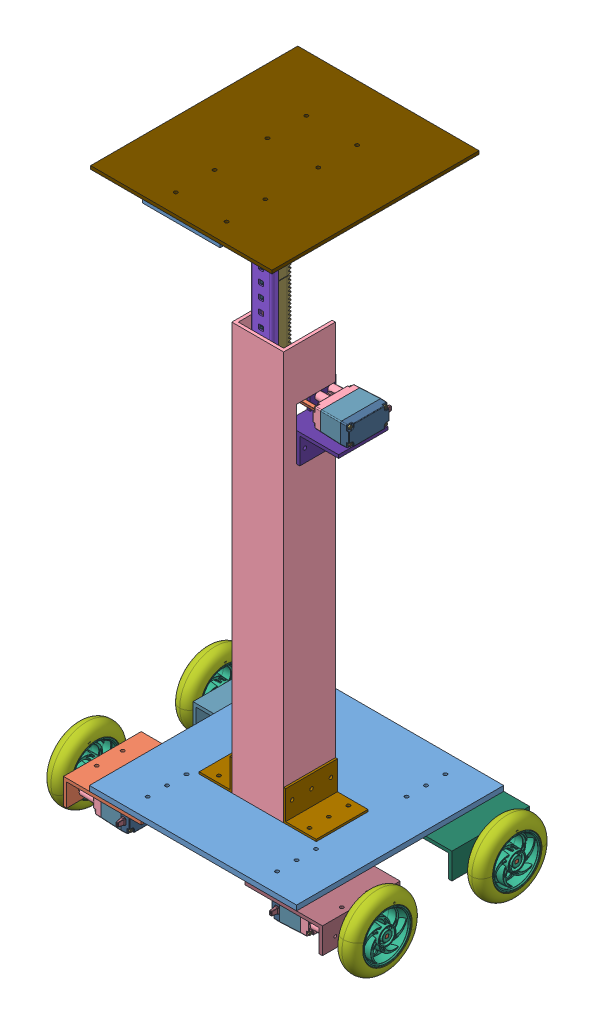
SolidWorks assembly mte380_Assy_01_lift_02., configuration Default. Lengths in mm.
Overall size (307.05 601.93 214.7).
138 component instances, 38 part files, 96 mates.
Components (placement in the parent):
- mte380_01_lift_base_02-1: mte380_01_lift_base_02 [Default] at (94.2351 110.2702 143.398) size (203.2 5 203.2)
- mte380_01_motor_bot_L_bracket_01-1: mte380_01_motor_bot_L_bracket_01 [Default] at (43.4351 110.2702 168.798) size (76.2 25.4 76.2)
- mte380_Assy_motor_vex_393_01-1: mte380_Assy_motor_vex_393_01 [Default] at (16.7501 95.0302 218.0279) x (0 0 -1) z (1 0 0) size (277.81 20.59 51.81)
  - SPPM206-0150BO-1: SPPM206-0150BO [Default] at (17.3 7.3 -1.5) x (1 0 0) z (0 -1 0) size (3.3 16.36 3.3)
  - 276-2181-003 Rev1-1: 276-2181-003 Rev1 [Default] at (0 0 -28) size (38.95 18.95 25.5)
  - 276-2177-019 Rev1-1: 276-2177-019 Rev1 [Default] at (-14.2702 0 -28) x (0.144195 -0.989549 0) z (0.989549 0.144195 0) size (6.3 15.8 6.3)
  - 276-2181-011 Rev1-1: 276-2181-011 Rev1 [Default] at (11.1298 0 -11) x (-1 0 0) z (0 1 0) size (11 4 11)
  - 276-2177-017 Rev1-1: 276-2177-017 Rev1 [Default] at (-245.51 0.1 2.5) size (248.21 15.59 2.54) (hidden)
  - QFK-N30QAV-16068-1: QFK-N30QAV-16068 [Default] at (-12.9 0 -23) x (0 1 0) z (0 0 1) size (12 10 26.1)
  - SPPM143-0030BO-1: SPPM143-0030BO [Default] at (-12.9 4.25 -6) x (-1 0 0) z (0 1 0) size (2.4 6.08 2.4)
  - 276-2181-010 Rev1-1: 276-2181-010 Rev1 [Default] at (10.8763 0 -9.4) x (0.878827 0.47714 0) z (0 0 1) size (1.5 1.5 16)
  - 276-2181-001 Rev1-1: 276-2181-001 Rev1 [Default] at origin size (40 20 8.01)
  - 276-2181-006 Rev1-1: 276-2181-006 Rev1 [Default] at (10.8763 0 -1.05) x (-0.259931 -0.965627 0) z (0 0 1) size (14.22 14.25 6.9)
  - 276-2181-007 Rev1-1: 276-2181-007 Rev1 [Default] at (2.1533 -1.4937 -4.4) x (-0.202497 0.979283 0) z (0 0 1) size (14.22 14.25 14.9)
  - 276-2181-010 Rev1-2: 276-2181-010 Rev1 [Default] at (-5.7003 2.586 -9.4) size (1.5 1.5 16)
  - 276-2177-018 Rev1-1: 276-2177-018 Rev1 [Default] at (-18.5 0.1 2.5) x (0 1 0) z (1 0 0) size (6.82 4.47 8.9)
  - 276-2181-006 Rev1-2: 276-2181-006 Rev1 [Default] at (2.1533 -1.4937 2.75) x (-0.071378 0.997449 0) z (0 0 1) size (14.22 14.25 6.9)
  - 276-2181-002 Rev1-1: 276-2181-002 Rev1 [Default] at (0 0 -20) size (40 20 23)
  - 276-2181-009 Rev1-1: 276-2181-009 Rev1 [Default] at (2.1533 -1.4937 -26.5) size (1.5 1.5 33)
  - SPPM206-0150BO-2: SPPM206-0150BO [Default] at (-16.9263 6.9263 -18.5) x (-0.075705 0.99713 0) z (-0.99713 -0.075705 0) size (3.3 16.36 3.3)
  - 276-2181-011 Rev1-2: 276-2181-011 Rev1 [Default] at (11.1298 0 -24) x (-0.997622 -0.068917 0) z (-0.068917 0.997622 0) size (11 4 11)
  - 276-2177-019 Rev1-2: 276-2177-019 Rev1 [Default] at (-1.5702 0 -28) x (0.32391 -0.946088 0) z (0.946088 0.32391 0) size (6.3 15.8 6.3)
  - SPPM206-0150BO-3: SPPM206-0150BO [Default] at (-17.3 -7.3 -1.5) x (0.292947 -0.956129 0) z (-0.956129 -0.292947 0) size (3.3 16.36 3.3)
  - SPPM206-0150BO-4: SPPM206-0150BO [Default] at (16.9263 -6.9263 -18.5) x (0.149257 -0.988799 0) z (0.988799 0.149257 0) size (3.3 16.36 3.3)
  - SPPM206-0150BO-5: SPPM206-0150BO [Default] at (17.3 -7.3 -1.5) x (1 0 0) z (0 -1 0) size (3.3 16.36 3.3)
  - SPPM206-0150BO-6: SPPM206-0150BO [Default] at (-16.9263 -6.9263 -18.5) x (-0.049887 0.998755 0) z (-0.998755 -0.049887 0) size (3.3 16.36 3.3)
  - SPPM206-0150BO-7: SPPM206-0150BO [Default] at (-17.3 7.3 -1.5) x (-0.963198 0.268794 0) z (0.268794 0.963198 0) size (3.3 16.36 3.3)
  - SPPM206-0150BO-8: SPPM206-0150BO [Default] at (16.9263 6.9263 -18.5) x (0.906825 0.421508 0) z (-0.421508 0.906825 0) size (3.3 16.36 3.3)
  - SPPM143-0030BO-2: SPPM143-0030BO [Default] at (-12.9 -4.25 -6) x (-0.988208 -0.153116 0) z (-0.153116 0.988208 0) size (2.4 6.08 2.4)
  - 276-2181-004 Rev1-1: 276-2181-004 Rev1 [Default] at (-12.9 0 -0.1) x (0.94341 -0.331628 0) z (0 0 -1) size (5.17 5.4 3)
  - 276-2181-005 Rev1-1: 276-2181-005 Rev1 [Default] at (-5.7003 2.586 -0.05) x (0.460478 -0.887671 0) z (0 0 1) size (11.88 11.88 5.9)
  - 276-2181-008 Rev1_276-2181-008g-1: 276-2181-008 Rev1_276-2181-008g [Default] at (11.1298 0 -14.5) x (0.267616 -0.963526 0) z (0 0 -1) size (13.83 13.88 17.3)
  - 276-2181-012 Rev1-1: 276-2181-012 Rev1 [Default] at (-12.9 0 -24) size (13.6 13 1)
- mte380_01_vex_shaft_2-1: mte380_01_vex_shaft_2 [Default] at (-31.9499 95.0479 206.9293) x (0 -0.267616 0.963526) z (-1 0 0) size (4.18 4.18 51.01)
- mte380_01_vex_bearing_block-1: mte380_01_vex_bearing_block [Default] at (-24.8662 107.0952 130.6495) x (0 0 -1) z (0 -1 0) size (35.56 10.16 13.39)
- mte380_01_center_shaft_01-1: mte380_01_center_shaft_01 [Default] at (68.8351 115.2702 130.698) size (50.8 400 50.8)
- mte380_Assy_wheel_vex_275-1: mte380_Assy_wheel_vex_275 [Default] at (-45.4869 83.9602 188.1506) x (0 0.267616 -0.963526) z (1 0 0) size (69.86 69.86 20.66)
  - SMALL-WHEEL-RIM-1: SMALL-WHEEL-RIM [Default] at (-15.1515 15.6838 -2.6601) size (61.43 61.43 9.24)
  - SMALL-WHEEL-HUB-1: SMALL-WHEEL-HUB [Default] at (-15.1515 15.6838 -2.6601) size (61.36 61.43 20.66)
  - SMALL-WHEEL-TIRE-1: SMALL-WHEEL-TIRE [Default] at (-15.1515 15.6838 -2.6601) x (1 0 0) z (0 -1 0) size (69.86 19.99 69.86)
- mte380_01_vex_rack_guide-1: mte380_01_vex_rack_guide [Default] at (94.2351 324.7702 178.323) x (-1 0 0) z (0 0 -1) size (20.84 444.5 8.8)
- mte380_01_vert_rack_bracket_01-1: mte380_01_vert_rack_bracket_01 [Default] at (119.6351 145.2702 130.698) size (32 30 50.8)
- mte380_01_vert_rack_bracket_01-2: mte380_01_vert_rack_bracket_01 [Default] at (68.8351 145.2702 181.498) x (-1 0 0) z (0 0 -1) size (32 30 50.8)
- mte380_01_vex_rack_slide-1: mte380_01_vex_rack_slide [Default] at (94.2351 558.9468 173.3216) x (1 0 0) z (0 1 0) size (17.45 8.37 50.79)
- mte380_01_vex_pinion_12-1: mte380_01_vex_pinion_12 [Default] at (93.7009 452.3921 151.0667) x (0 0.267616 -0.963526) z (1 0 0) size (14.8 14.8 9.53)
- mte380_01_vex_rack-1: mte380_01_vex_rack [Default] at (94.2351 590.6968 168.7501) x (0 1 0) z (-1 0 0) size (63 14.6 12.7)
- mte380_01_vex_rack_slide-2: mte380_01_vex_rack_slide [Default] at (94.2351 622.4468 173.3216) x (1 0 0) z (0 1 0) size (17.45 8.37 50.79)
- mte380_01_motor_bot_R_bracket_01-1: mte380_01_motor_bot_R_bracket_01 [Default] at (145.0351 110.2702 244.998) x (-1 0 0) z (0 0 -1) size (76.2 25.4 76.2)
- mte380_Assy_motor_vex_393_01-2: mte380_Assy_motor_vex_393_01 [Default] at (172.3201 95.0302 218.0279) x (0 0 -1) z (-1 0 0) size (277.81 20.59 51.81)
  - SPPM206-0150BO-1: SPPM206-0150BO [Default] at (17.3 7.3 -1.5) x (1 0 0) z (0 -1 0) size (3.3 16.36 3.3)
  - 276-2181-003 Rev1-1: 276-2181-003 Rev1 [Default] at (0 0 -28) size (38.95 18.95 25.5)
  - 276-2177-019 Rev1-1: 276-2177-019 Rev1 [Default] at (-14.2702 0 -28) x (0.144195 -0.989549 0) z (0.989549 0.144195 0) size (6.3 15.8 6.3)
  - 276-2181-011 Rev1-1: 276-2181-011 Rev1 [Default] at (11.1298 0 -11) x (-1 0 0) z (0 1 0) size (11 4 11)
  - 276-2177-017 Rev1-1: 276-2177-017 Rev1 [Default] at (-245.51 0.1 2.5) size (248.21 15.59 2.54) (hidden)
  - QFK-N30QAV-16068-1: QFK-N30QAV-16068 [Default] at (-12.9 0 -23) x (0 1 0) z (0 0 1) size (12 10 26.1)
  - SPPM143-0030BO-1: SPPM143-0030BO [Default] at (-12.9 4.25 -6) x (-1 0 0) z (0 1 0) size (2.4 6.08 2.4)
  - 276-2181-010 Rev1-1: 276-2181-010 Rev1 [Default] at (10.8763 0 -9.4) x (0.878827 0.47714 0) z (0 0 1) size (1.5 1.5 16)
  - 276-2181-001 Rev1-1: 276-2181-001 Rev1 [Default] at origin size (40 20 8.01)
  - 276-2181-006 Rev1-1: 276-2181-006 Rev1 [Default] at (10.8763 0 -1.05) x (-0.259931 -0.965627 0) z (0 0 1) size (14.22 14.25 6.9)
  - 276-2181-007 Rev1-1: 276-2181-007 Rev1 [Default] at (2.1533 -1.4937 -4.4) x (-0.202497 0.979283 0) z (0 0 1) size (14.22 14.25 14.9)
  - 276-2181-010 Rev1-2: 276-2181-010 Rev1 [Default] at (-5.7003 2.586 -9.4) size (1.5 1.5 16)
  - 276-2177-018 Rev1-1: 276-2177-018 Rev1 [Default] at (-18.5 0.1 2.5) x (0 1 0) z (1 0 0) size (6.82 4.47 8.9)
  - 276-2181-006 Rev1-2: 276-2181-006 Rev1 [Default] at (2.1533 -1.4937 2.75) x (-0.071378 0.997449 0) z (0 0 1) size (14.22 14.25 6.9)
  - 276-2181-002 Rev1-1: 276-2181-002 Rev1 [Default] at (0 0 -20) size (40 20 23)
  - 276-2181-009 Rev1-1: 276-2181-009 Rev1 [Default] at (2.1533 -1.4937 -26.5) size (1.5 1.5 33)
  - SPPM206-0150BO-2: SPPM206-0150BO [Default] at (-16.9263 6.9263 -18.5) x (-0.075705 0.99713 0) z (-0.99713 -0.075705 0) size (3.3 16.36 3.3)
  - 276-2181-011 Rev1-2: 276-2181-011 Rev1 [Default] at (11.1298 0 -24) x (-0.997622 -0.068917 0) z (-0.068917 0.997622 0) size (11 4 11)
  - 276-2177-019 Rev1-2: 276-2177-019 Rev1 [Default] at (-1.5702 0 -28) x (0.32391 -0.946088 0) z (0.946088 0.32391 0) size (6.3 15.8 6.3)
  - SPPM206-0150BO-3: SPPM206-0150BO [Default] at (-17.3 -7.3 -1.5) x (0.292947 -0.956129 0) z (-0.956129 -0.292947 0) size (3.3 16.36 3.3)
  - SPPM206-0150BO-4: SPPM206-0150BO [Default] at (16.9263 -6.9263 -18.5) x (0.149257 -0.988799 0) z (0.988799 0.149257 0) size (3.3 16.36 3.3)
  - SPPM206-0150BO-5: SPPM206-0150BO [Default] at (17.3 -7.3 -1.5) x (1 0 0) z (0 -1 0) size (3.3 16.36 3.3)
  - SPPM206-0150BO-6: SPPM206-0150BO [Default] at (-16.9263 -6.9263 -18.5) x (-0.049887 0.998755 0) z (-0.998755 -0.049887 0) size (3.3 16.36 3.3)
  - SPPM206-0150BO-7: SPPM206-0150BO [Default] at (-17.3 7.3 -1.5) x (-0.963198 0.268794 0) z (0.268794 0.963198 0) size (3.3 16.36 3.3)
  - SPPM206-0150BO-8: SPPM206-0150BO [Default] at (16.9263 6.9263 -18.5) x (0.906825 0.421508 0) z (-0.421508 0.906825 0) size (3.3 16.36 3.3)
  - SPPM143-0030BO-2: SPPM143-0030BO [Default] at (-12.9 -4.25 -6) x (-0.988208 -0.153116 0) z (-0.153116 0.988208 0) size (2.4 6.08 2.4)
  - 276-2181-004 Rev1-1: 276-2181-004 Rev1 [Default] at (-12.9 0 -0.1) x (0.94341 -0.331628 0) z (0 0 -1) size (5.17 5.4 3)
  - 276-2181-005 Rev1-1: 276-2181-005 Rev1 [Default] at (-5.7003 2.586 -0.05) x (0.460478 -0.887671 0) z (0 0 1) size (11.88 11.88 5.9)
  - 276-2181-008 Rev1_276-2181-008g-1: 276-2181-008 Rev1_276-2181-008g [Default] at (11.1298 0 -14.5) x (0.267616 -0.963526 0) z (0 0 -1) size (13.83 13.88 17.3)
  - 276-2181-012 Rev1-1: 276-2181-012 Rev1 [Default] at (-12.9 0 -24) size (13.6 13 1)
- mte380_01_vex_shaft_2-2: mte380_01_vex_shaft_2 [Default] at (221.0201 95.0615 206.9157) x (0 0.267616 0.963526) z (-1 0 0) size (4.18 4.18 51.01)
- mte380_Assy_wheel_vex_275-4: mte380_Assy_wheel_vex_275 [Default] at (239.8772 75.9124 196.4833) x (0 -0.267616 -0.963526) z (1 0 0) size (69.86 69.86 20.66)
  - SMALL-WHEEL-RIM-1: SMALL-WHEEL-RIM [Default] at (-15.1515 15.6838 -2.6601) size (61.43 61.43 9.24)
  - SMALL-WHEEL-HUB-1: SMALL-WHEEL-HUB [Default] at (-15.1515 15.6838 -2.6601) size (61.36 61.43 20.66)
  - SMALL-WHEEL-TIRE-1: SMALL-WHEEL-TIRE [Default] at (-15.1515 15.6838 -2.6601) x (1 0 0) z (0 -1 0) size (69.86 19.99 69.86)
- mte380_01_vex_shaft_2-3: mte380_01_vex_shaft_2 [Default] at (221.2351 95.0937 79.8345) x (0 0 1) z (-1 0 0) size (4.18 4.18 51.01)
- mte380_01_vex_shaft_2-4: mte380_01_vex_shaft_2 [Default] at (-32.7649 95.1912 79.8345) x (0 0 1) z (-1 0 0) size (4.18 4.18 51.01)
- mte380_01_front_bot_L_bracket_01-1: mte380_01_front_bot_L_bracket_01 [Default] at (43.4351 110.2702 41.798) size (76.2 25.4 76.2)
- mte380_01_front_bot_R_bracket_01-1: mte380_01_front_bot_R_bracket_01 [Default] at (145.0351 110.2702 117.998) x (-1 0 0) z (0 0 -1) size (76.2 25.4 76.2)
- mte380_01_vex_flat_bearing-2: mte380_01_vex_flat_bearing [Default] at (129.0839 107.7302 106.314) x (1 0 0) z (0 1 0) size (7.04 35.56 10.16)
- mte380_01_vex_flat_bearing-3: mte380_01_vex_flat_bearing [Default] at (59.3863 107.7302 53.482) x (-1 0 0) z (0 1 0) size (7.04 35.56 10.16)
- mte380_Assy_wheel_vex_275-5: mte380_Assy_wheel_vex_275 [Default] at (-46.3019 79.4824 64.708) x (0 0 -1) z (1 0 0) size (69.86 69.86 20.66)
  - SMALL-WHEEL-RIM-1: SMALL-WHEEL-RIM [Default] at (-15.1515 15.6838 -2.6601) size (61.43 61.43 9.24)
  - SMALL-WHEEL-HUB-1: SMALL-WHEEL-HUB [Default] at (-15.1515 15.6838 -2.6601) size (61.36 61.43 20.66)
  - SMALL-WHEEL-TIRE-1: SMALL-WHEEL-TIRE [Default] at (-15.1515 15.6838 -2.6601) x (1 0 0) z (0 -1 0) size (69.86 19.99 69.86)
- mte380_Assy_wheel_vex_275-6: mte380_Assy_wheel_vex_275 [Default] at (240.0922 79.4349 64.658) x (0 0 -1) z (1 0 0) size (69.86 69.86 20.66)
  - SMALL-WHEEL-RIM-1: SMALL-WHEEL-RIM [Default] at (-15.1515 15.6838 -2.6601) size (61.43 61.43 9.24)
  - SMALL-WHEEL-HUB-1: SMALL-WHEEL-HUB [Default] at (-15.1515 15.6838 -2.6601) size (61.36 61.43 20.66)
  - SMALL-WHEEL-TIRE-1: SMALL-WHEEL-TIRE [Default] at (-15.1515 15.6838 -2.6601) x (1 0 0) z (0 -1 0) size (69.86 19.99 69.86)
- mte380_01_pinion_motor_mount_01-1: mte380_01_pinion_motor_mount_01 [Default] at (122.8101 413.6702 168.798) x (-1 0 0) z (0 0 -1) size (53.98 47.63 48.26)
- mte380_Assy_motor_vex_393_01-3: mte380_Assy_motor_vex_393_01 [Default] at (153.9101 452.4052 139.8882) x (0 0 1) z (1 0 0) size (277.81 20.59 51.81)
  - SPPM206-0150BO-1: SPPM206-0150BO [Default] at (17.3 7.3 -1.5) x (1 0 0) z (0 -1 0) size (3.3 16.36 3.3)
  - 276-2181-003 Rev1-1: 276-2181-003 Rev1 [Default] at (0 0 -28) size (38.95 18.95 25.5)
  - 276-2177-019 Rev1-1: 276-2177-019 Rev1 [Default] at (-14.2702 0 -28) x (0.144195 -0.989549 0) z (0.989549 0.144195 0) size (6.3 15.8 6.3)
  - 276-2181-011 Rev1-1: 276-2181-011 Rev1 [Default] at (11.1298 0 -11) x (-1 0 0) z (0 1 0) size (11 4 11)
  - 276-2177-017 Rev1-1: 276-2177-017 Rev1 [Default] at (-245.51 0.1 2.5) size (248.21 15.59 2.54) (hidden)
  - QFK-N30QAV-16068-1: QFK-N30QAV-16068 [Default] at (-12.9 0 -23) x (0 1 0) z (0 0 1) size (12 10 26.1)
  - SPPM143-0030BO-1: SPPM143-0030BO [Default] at (-12.9 4.25 -6) x (-1 0 0) z (0 1 0) size (2.4 6.08 2.4)
  - 276-2181-010 Rev1-1: 276-2181-010 Rev1 [Default] at (10.8763 0 -9.4) x (0.878827 0.47714 0) z (0 0 1) size (1.5 1.5 16)
  - 276-2181-001 Rev1-1: 276-2181-001 Rev1 [Default] at origin size (40 20 8.01)
  - 276-2181-006 Rev1-1: 276-2181-006 Rev1 [Default] at (10.8763 0 -1.05) x (-0.259931 -0.965627 0) z (0 0 1) size (14.22 14.25 6.9)
  - 276-2181-007 Rev1-1: 276-2181-007 Rev1 [Default] at (2.1533 -1.4937 -4.4) x (-0.202497 0.979283 0) z (0 0 1) size (14.22 14.25 14.9)
  - 276-2181-010 Rev1-2: 276-2181-010 Rev1 [Default] at (-5.7003 2.586 -9.4) size (1.5 1.5 16)
  - 276-2177-018 Rev1-1: 276-2177-018 Rev1 [Default] at (-18.5 0.1 2.5) x (0 1 0) z (1 0 0) size (6.82 4.47 8.9)
  - 276-2181-006 Rev1-2: 276-2181-006 Rev1 [Default] at (2.1533 -1.4937 2.75) x (-0.071378 0.997449 0) z (0 0 1) size (14.22 14.25 6.9)
  - 276-2181-002 Rev1-1: 276-2181-002 Rev1 [Default] at (0 0 -20) size (40 20 23)
  - 276-2181-009 Rev1-1: 276-2181-009 Rev1 [Default] at (2.1533 -1.4937 -26.5) size (1.5 1.5 33)
  - SPPM206-0150BO-2: SPPM206-0150BO [Default] at (-16.9263 6.9263 -18.5) x (-0.075705 0.99713 0) z (-0.99713 -0.075705 0) size (3.3 16.36 3.3)
  - 276-2181-011 Rev1-2: 276-2181-011 Rev1 [Default] at (11.1298 0 -24) x (-0.997622 -0.068917 0) z (-0.068917 0.997622 0) size (11 4 11)
  - 276-2177-019 Rev1-2: 276-2177-019 Rev1 [Default] at (-1.5702 0 -28) x (0.32391 -0.946088 0) z (0.946088 0.32391 0) size (6.3 15.8 6.3)
  - SPPM206-0150BO-3: SPPM206-0150BO [Default] at (-17.3 -7.3 -1.5) x (0.292947 -0.956129 0) z (-0.956129 -0.292947 0) size (3.3 16.36 3.3)
  - SPPM206-0150BO-4: SPPM206-0150BO [Default] at (16.9263 -6.9263 -18.5) x (0.149257 -0.988799 0) z (0.988799 0.149257 0) size (3.3 16.36 3.3)
  - SPPM206-0150BO-5: SPPM206-0150BO [Default] at (17.3 -7.3 -1.5) x (1 0 0) z (0 -1 0) size (3.3 16.36 3.3)
  - SPPM206-0150BO-6: SPPM206-0150BO [Default] at (-16.9263 -6.9263 -18.5) x (-0.049887 0.998755 0) z (-0.998755 -0.049887 0) size (3.3 16.36 3.3)
  - SPPM206-0150BO-7: SPPM206-0150BO [Default] at (-17.3 7.3 -1.5) x (-0.963198 0.268794 0) z (0.268794 0.963198 0) size (3.3 16.36 3.3)
  - SPPM206-0150BO-8: SPPM206-0150BO [Default] at (16.9263 6.9263 -18.5) x (0.906825 0.421508 0) z (-0.421508 0.906825 0) size (3.3 16.36 3.3)
  - SPPM143-0030BO-2: SPPM143-0030BO [Default] at (-12.9 -4.25 -6) x (-0.988208 -0.153116 0) z (-0.153116 0.988208 0) size (2.4 6.08 2.4)
  - 276-2181-004 Rev1-1: 276-2181-004 Rev1 [Default] at (-12.9 0 -0.1) x (0.94341 -0.331628 0) z (0 0 -1) size (5.17 5.4 3)
  - 276-2181-005 Rev1-1: 276-2181-005 Rev1 [Default] at (-5.7003 2.586 -0.05) x (0.460478 -0.887671 0) z (0 0 1) size (11.88 11.88 5.9)
  - 276-2181-008 Rev1_276-2181-008g-1: 276-2181-008 Rev1_276-2181-008g [Default] at (11.1298 0 -14.5) x (0.267616 -0.963526 0) z (0 0 -1) size (13.83 13.88 17.3)
  - 276-2181-012 Rev1-1: 276-2181-012 Rev1 [Default] at (-12.9 0 -24) size (13.6 13 1)
- mte380_01_vex_shaft_2-5: mte380_01_vex_shaft_2 [Default] at (105.2101 452.4229 151.0493) x (0 -0.267616 0.963526) z (-1 0 0) size (4.18 4.18 51.01)
- mte380_01_lift_platform_02-1: mte380_01_lift_platform_02 [Default] at (183.1351 650.7718 53.298) size (177.8 3.17 203.2)
- mte380_01_lift_platform__bracket_01-1: mte380_01_lift_platform__bracket_01 [Default] at (132.3351 622.1968 168.7501) x (0 0 1) z (-1 0 0) size (79.38 28.57 76.2)
- mte380_01_lift_platform__bracket_01-2: mte380_01_lift_platform__bracket_01 [Default] at (56.1351 622.1968 177.123) x (0 0 -1) z (1 0 0) size (79.38 28.57 76.2)
- mte380_01_vex_rack_slide-3: mte380_01_vex_rack_slide [Default] at (94.2351 431.9468 173.3216) x (1 0 0) z (0 1 0) size (17.45 8.37 50.79)
- mte380_01_vex_rack-2: mte380_01_vex_rack [Default] at (94.2351 463.6968 168.7501) x (0 1 0) z (-1 0 0) size (63 14.6 12.7)
- mte380_01_vex_rack_slide-4: mte380_01_vex_rack_slide [Default] at (94.2351 495.4468 173.3216) x (1 0 0) z (0 1 0) size (17.45 8.37 50.79)
- mte380_01_vex_rack-3: mte380_01_vex_rack [Default] at (94.2351 527.1968 168.7501) x (0 1 0) z (-1 0 0) size (63 14.6 12.7)
Mates (geometry in assembly coordinates):
- Coincident2: coincident: line of mte380_01_lift_base_02-1 through (-7.3649 110.2702 244.998) axis (1 0 0); plane of mte380_01_motor_bot_L_bracket_01-1 through (43.4351 110.2702 244.998) normal (0 0 1)
- Coincident7: coincident anti-aligned: plane of mte380_Assy_motor_vex_393_01-1/276-2181-008 Rev1_276-2181-008g-1 through (-6.5499 96.1526 208.8837) normal (0 0.267616 -0.963526); plane of mte380_01_vex_shaft_2-1 through (-57.3499 93.0935 208.034) normal (0 -0.267616 0.963526)
- Coincident8: coincident anti-aligned: plane of mte380_Assy_motor_vex_393_01-1/276-2181-008 Rev1_276-2181-008g-1 through (-6.5499 97.0159 205.7756) normal (0 -0.963526 -0.267616); plane of mte380_01_vex_shaft_2-1 through (-57.3499 97.0023 205.8245) normal (0 0.963526 0.267616)
- Coincident9: coincident anti-aligned: plane of mte380_Assy_motor_vex_393_01-1/276-2181-008 Rev1_276-2181-008g-1 through (-6.5499 93.0445 208.0204) normal (-1 0 0); plane of mte380_01_vex_shaft_2-1 through (-6.5499 97.0023 205.8245) normal (1 0 0)
- Coincident10: coincident anti-aligned: plane of mte380_01_lift_base_02-1 through (94.2351 110.2702 143.398) normal (0 -1 0); plane of mte380_01_motor_bot_L_bracket_01-1 through (43.4351 110.2702 244.998) normal (0 1 0)
- Coincident29: coincident aligned: plane of mte380_01_lift_base_02-1 through (-7.3649 115.2702 244.998) normal (0 0 1); plane of mte380_01_motor_bot_L_bracket_01-1 through (43.4351 110.2702 244.998) normal (0 0 1)
- Distance3: distance = 50.8 mm anti-aligned: plane of mte380_01_lift_base_02-1 through (-7.3649 115.2702 244.998) normal (-1 0 0); plane of mte380_01_motor_bot_L_bracket_01-1 through (43.4351 107.0952 244.998) normal (1 0 0)
- Distance5: distance = 2.54 mm anti-aligned: plane of mte380_Assy_motor_vex_393_01-1/276-2177-019 Rev1-2 through (-27.0499 95.0302 219.598) normal (-1 0 0); plane of mte380_01_motor_bot_L_bracket_01-1 through (-29.5899 84.8702 244.998) normal (1 0 0)
- Coincident48: coincident anti-aligned: plane of mte380_01_lift_base_02-1 through (94.2351 115.2702 143.398) normal (0 1 0); plane of mte380_01_center_shaft_01-1 through (68.8351 115.2702 130.698) normal (0 -1 0)
- Width1: width anti-aligned: plane of mte380_01_lift_base_02-1 through (-7.3649 115.2702 244.998) normal (-1 0 0); plane of mte380_01_lift_base_02-1 through (195.8351 115.2702 244.998) normal (1 0 0); plane of mte380_01_center_shaft_01-1 through (119.6351 515.2702 181.498) normal (1 0 0); plane of mte380_01_center_shaft_01-1 through (68.8351 515.2702 130.698) normal (-1 0 0)
- Distance6: distance = 63.5 mm aligned: plane of mte380_01_center_shaft_01-1 through (68.8351 515.2702 181.498) normal (0 0 1); plane of mte380_01_lift_base_02-1 through (-7.3649 115.2702 244.998) normal (0 0 1)
- Coincident52: coincident anti-aligned: plane of mte380_01_vex_shaft_2-1 through (-57.3499 93.9431 204.9748) normal (0 0.267616 -0.963526); plane of mte380_Assy_wheel_vex_275-1/SMALL-WHEEL-HUB-1 through (-36.717 93.895 204.9615) normal (0 -0.267616 0.963526)
- Coincident53: coincident anti-aligned: plane of mte380_01_vex_shaft_2-1 through (-57.3499 97.0023 205.8245) normal (0 0.963526 0.267616); plane of mte380_Assy_wheel_vex_275-1/SMALL-WHEEL-HUB-1 through (-36.717 97.0023 205.8245) normal (0 -0.963526 -0.267616)
- Tangent9: tangent anti-aligned: plane of mte380_01_vex_shaft_2-1 through (-57.3499 97.0023 205.8245) normal (-1 0 0); sphere of mte380_Assy_wheel_vex_275-1/SMALL-WHEEL-HUB-1
- Coincident55: coincident anti-aligned: plane of mte380_01_center_shaft_01-1 through (116.4601 515.2702 178.323) normal (0 0 -1); plane of mte380_01_vex_rack_guide-1 through (85.7693 172.3702 178.323) normal (0 0 1)
- Width2: width anti-aligned: plane of mte380_01_center_shaft_01-1 through (116.4601 515.2702 130.698) normal (-1 0 0); plane of mte380_01_center_shaft_01-1 through (72.0101 515.2702 178.323) normal (1 0 0); plane of mte380_01_vex_rack_guide-1 through (104.59 172.3702 175.861) normal (0.965926 0 -0.258819); plane of mte380_01_vex_rack_guide-1 through (85.5782 172.3702 169.5238) normal (-0.965926 0 -0.258819)
- Coincident56: coincident anti-aligned: plane of mte380_01_center_shaft_01-1 through (119.6351 515.2702 181.498) normal (1 0 0); plane of mte380_01_vert_rack_bracket_01-1 through (119.6351 145.2702 181.498) normal (-1 0 0)
- Coincident57: coincident anti-aligned: plane of mte380_01_lift_base_02-1 through (94.2351 115.2702 143.398) normal (0 1 0); plane of mte380_01_vert_rack_bracket_01-1 through (119.6351 115.2702 181.498) normal (0 -1 0)
- Coincident58: coincident anti-aligned: plane of mte380_01_center_shaft_01-1 through (68.8351 515.2702 130.698) normal (-1 0 0); plane of mte380_01_vert_rack_bracket_01-2 through (68.8351 145.2702 130.698) normal (1 0 0)
- Coincident59: coincident anti-aligned: plane of mte380_01_lift_base_02-1 through (94.2351 115.2702 143.398) normal (0 1 0); plane of mte380_01_vert_rack_bracket_01-2 through (68.8351 115.2702 130.698) normal (0 -1 0)
- Coincident61: coincident anti-aligned: plane of mte380_01_vex_rack_guide-1 through (102.7008 172.3702 177.123) normal (0 0 -1); plane of mte380_01_vex_rack_slide-1 through (94.2351 558.9468 177.123) normal (0 0 1)
- Width3: width anti-aligned: plane of mte380_01_vex_rack_slide-1 through (103.5283 584.3468 177.2489) normal (0.965926 0 -0.258819); plane of mte380_01_vex_rack_slide-1 through (87.0326 584.3468 169.446) normal (-0.965926 0 -0.258819); plane of mte380_01_vex_rack_guide-1 through (101.7328 172.3702 169.8344) normal (-0.965926 0 0.258819); plane of mte380_01_vex_rack_guide-1 through (85.0393 172.3702 176.1716) normal (0.965926 0 0.258819)
- Coincident63: coincident anti-aligned: plane of mte380_01_vex_rack_slide-1 through (101.5342 584.3468 168.7501) normal (0 0 -1); plane of mte380_01_vex_rack-1 through (94.2351 590.6968 168.7501) normal (0 0 1)
- Coincident64: coincident anti-aligned: plane of mte380_01_vex_rack_guide-1 through (102.7008 172.3702 177.123) normal (0 0 -1); plane of mte380_01_vex_rack_slide-2 through (94.2351 622.4468 177.123) normal (0 0 1)
- Width4: width anti-aligned: plane of mte380_01_vex_rack_slide-2 through (103.5283 647.8468 177.2489) normal (0.965926 0 -0.258819); plane of mte380_01_vex_rack_slide-2 through (87.0326 647.8468 169.446) normal (-0.965926 0 -0.258819); plane of mte380_01_vex_rack_guide-1 through (101.7328 172.3702 169.8344) normal (-0.965926 0 0.258819); plane of mte380_01_vex_rack_guide-1 through (85.0393 172.3702 176.1716) normal (0.965926 0 0.258819)
- Concentric9: concentric anti-aligned: cylinder of mte380_01_vex_rack_slide-1 through (94.2351 565.2968 168.7501) axis (0 0 -1) radius 1.85; cylinder of mte380_01_vex_rack-1 through (94.2351 565.2968 168.7501) axis (0 0 1) radius 2.25
- Concentric12: concentric anti-aligned: cylinder of mte380_01_vex_rack-1 through (94.2351 616.0968 168.7501) axis (0 0 1) radius 2.25; cylinder of mte380_01_vex_rack_slide-2 through (94.2351 616.0968 168.7501) axis (0 0 -1) radius 1.85
- Coincident65: coincident aligned: plane of mte380_01_center_shaft_01-1 through (119.6351 515.2702 130.698) normal (0 0 -1); plane of mte380_01_vert_rack_bracket_01-1 through (119.6351 145.2702 130.698) normal (0 0 -1)
- Coincident66: coincident aligned: plane of mte380_01_center_shaft_01-1 through (72.0101 515.2702 130.698) normal (0 0 -1); plane of mte380_01_vert_rack_bracket_01-2 through (68.8351 145.2702 130.698) normal (0 0 -1)
- Coincident67: coincident anti-aligned: plane of mte380_01_lift_base_02-1 through (94.2351 110.2702 143.398) normal (0 -1 0); plane of mte380_01_motor_bot_R_bracket_01-1 through (145.0351 110.2702 168.798) normal (0 1 0)
- Coincident68: coincident aligned: plane of mte380_01_lift_base_02-1 through (-7.3649 115.2702 244.998) normal (0 0 1); plane of mte380_01_motor_bot_R_bracket_01-1 through (145.0351 110.2702 244.998) normal (0 0 1)
- Distance7: distance = 50.8 mm: line of mte380_01_lift_base_02-1 through (195.8351 115.2702 244.998) axis (0 -1 0); line of mte380_01_motor_bot_R_bracket_01-1 through (145.0351 107.0952 244.998) axis (0 1 0)
- Concentric13: concentric aligned: cylinder of mte380_01_motor_bot_R_bracket_01-1 through (221.2351 95.0302 219.598) axis (1 0 0) radius 1.3526; cylinder of mte380_Assy_motor_vex_393_01-2/276-2177-019 Rev1-2 through (216.1201 95.0302 219.598) axis (1 0 0) radius 1.3526
- Concentric14: concentric aligned: cylinder of mte380_01_motor_bot_R_bracket_01-1 through (221.2351 95.0302 232.298) axis (1 0 0) radius 1.3526; cylinder of mte380_Assy_motor_vex_393_01-2/276-2177-019 Rev1-1 through (216.1201 95.0302 232.298) axis (1 0 0) radius 1.3526
- Distance8: distance = 2.54 mm anti-aligned: plane of mte380_Assy_motor_vex_393_01-2/276-2181-003 Rev1-1 through (215.5201 95.0302 218.0279) normal (1 0 0); plane of mte380_01_motor_bot_R_bracket_01-1 through (218.0601 84.8702 168.798) normal (-1 0 0)
- Coincident71: coincident anti-aligned: plane of mte380_Assy_motor_vex_393_01-2/276-2181-008 Rev1_276-2181-008g-1 through (195.6201 97.0159 208.0204) normal (1 0 0); plane of mte380_01_vex_shaft_2-2 through (195.6201 96.1662 204.9613) normal (-1 0 0)
- Coincident72: coincident anti-aligned: plane of mte380_Assy_motor_vex_393_01-2/276-2181-008 Rev1_276-2181-008g-1 through (195.6201 96.1526 204.9123) normal (0 -0.963526 0.267616); plane of mte380_01_vex_shaft_2-2 through (195.6201 96.1662 204.9613) normal (0 0.963526 -0.267616)
- Coincident73: coincident anti-aligned: plane of mte380_Assy_motor_vex_393_01-2/276-2181-008 Rev1_276-2181-008g-1 through (195.6201 93.9078 208.8837) normal (0 -0.267616 -0.963526); plane of mte380_01_vex_shaft_2-2 through (195.6201 93.9567 208.8701) normal (0 0.267616 0.963526)
- Coincident74: coincident anti-aligned: plane of mte380_01_vex_shaft_2-2 through (195.6201 93.107 205.8109) normal (0 -0.963526 0.267616); plane of mte380_Assy_wheel_vex_275-4/SMALL-WHEEL-HUB-1 through (248.6472 93.9567 208.8701) normal (0 0.963526 -0.267616)
- Coincident76: coincident anti-aligned: plane of mte380_01_vex_shaft_2-2 through (195.6201 93.9567 208.8701) normal (0 0.267616 0.963526); plane of mte380_Assy_wheel_vex_275-4/SMALL-WHEEL-HUB-1 through (248.6472 97.0641 208.0071) normal (0 -0.267616 -0.963526)
- Tangent11: tangent anti-aligned: plane of mte380_01_vex_shaft_2-2 through (246.4201 96.1662 204.9613) normal (1 0 0); sphere of mte380_Assy_wheel_vex_275-4/SMALL-WHEEL-HUB-1
- Concentric17: concentric anti-aligned: cylinder of mte380_01_motor_bot_L_bracket_01-1 through (-25.5934 110.2702 219.598) axis (0 1 0) radius 1.7272; cone of mte380_01_vex_bearing_block-1 through (-25.5934 107.0952 219.598) axis (0 -1 0)
- Distance13: distance = 0 mm anti-aligned: plane of mte380_01_vex_bearing_block-1 through (-31.6896 107.0952 228.2341) normal (0 1 0); plane of mte380_01_motor_bot_L_bracket_01-1 through (-29.5899 107.0952 244.998) normal (0 -1 0)
- Concentric18: concentric aligned: cylinder of mte380_01_motor_bot_L_bracket_01-1 through (-32.7649 95.0302 232.298) axis (-1 0 0) radius 1.3526; circle of mte380_Assy_motor_vex_393_01-1/276-2177-019 Rev1-1
- Concentric19: concentric aligned: circle of mte380_01_motor_bot_L_bracket_01-1; circle of mte380_Assy_motor_vex_393_01-1/276-2177-019 Rev1-2
- Coincident99: coincident anti-aligned: plane of mte380_01_lift_base_02-1 through (94.2351 110.2702 143.398) normal (0 -1 0); plane of mte380_01_front_bot_L_bracket_01-1 through (43.4351 110.2702 117.998) normal (0 1 0)
- Coincident100: coincident aligned: plane of mte380_01_lift_base_02-1 through (-7.3649 115.2702 41.798) normal (0 0 -1); plane of mte380_01_front_bot_L_bracket_01-1 through (43.4351 110.2702 41.798) normal (0 0 -1)
- Distance14: distance = 50.8 mm anti-aligned: plane of mte380_01_front_bot_L_bracket_01-1 through (43.4351 107.0952 117.998) normal (1 0 0); plane of mte380_01_lift_base_02-1 through (-7.3649 115.2702 244.998) normal (-1 0 0)
- Coincident102: coincident anti-aligned: plane of mte380_01_lift_base_02-1 through (94.2351 110.2702 143.398) normal (0 -1 0); plane of mte380_01_front_bot_R_bracket_01-1 through (145.0351 110.2702 41.798) normal (0 1 0)
- Coincident103: coincident aligned: plane of mte380_01_lift_base_02-1 through (-7.3649 115.2702 41.798) normal (0 0 -1); plane of mte380_01_front_bot_R_bracket_01-1 through (145.0351 110.2702 41.798) normal (0 0 -1)
- Distance16: distance = 50.8 mm anti-aligned: plane of mte380_01_front_bot_R_bracket_01-1 through (145.0351 107.0952 41.798) normal (-1 0 0); plane of mte380_01_lift_base_02-1 through (195.8351 115.2702 244.998) normal (1 0 0)
- Concentric20: concentric anti-aligned: cylinder of mte380_01_front_bot_R_bracket_01-1 through (221.2351 95.0302 67.198) axis (1 0 0) radius 1.7272; circle of mte380_01_vex_flat_bearing-2
- Coincident106: coincident anti-aligned: plane of mte380_01_front_bot_R_bracket_01-1 through (218.0601 84.8702 41.798) normal (-1 0 0); plane of mte380_01_vex_flat_bearing-2 through (218.0601 107.7302 106.314) normal (1 0 0)
- Concentric21: concentric anti-aligned: circle of mte380_01_front_bot_R_bracket_01-1; cylinder of mte380_01_vex_flat_bearing-2 through (211.7101 95.0302 92.598) axis (-1 0 0) radius 2.1209
- Concentric22: concentric anti-aligned: cylinder of mte380_01_front_bot_L_bracket_01-1 through (-32.7649 95.0302 67.198) axis (-1 0 0) radius 1.7272; cylinder of mte380_01_vex_flat_bearing-3 through (-23.2399 95.0302 67.198) axis (1 0 0) radius 2.1209
- Concentric23: concentric anti-aligned: cylinder of mte380_01_front_bot_L_bracket_01-1 through (-32.7649 95.0302 92.598) axis (-1 0 0) radius 1.7272; cylinder of mte380_01_vex_flat_bearing-3 through (-23.2399 95.0302 92.598) axis (1 0 0) radius 2.1209
- Coincident107: coincident anti-aligned: plane of mte380_01_front_bot_L_bracket_01-1 through (-29.5899 84.8702 117.998) normal (1 0 0); plane of mte380_01_vex_flat_bearing-3 through (-29.5899 107.7302 53.482) normal (-1 0 0)
- Coincident108: coincident anti-aligned: plane of mte380_01_vex_shaft_2-4 through (-58.1649 93.6037 78.247) normal (0 0 -1); plane of mte380_Assy_wheel_vex_275-5/SMALL-WHEEL-HUB-1 through (-37.532 93.5537 78.247) normal (0 0 1)
- Coincident109: coincident anti-aligned: plane of mte380_01_vex_shaft_2-4 through (-58.1649 96.7787 78.247) normal (0 1 0); plane of ? through (-37.532 96.7787 78.247) normal (0 -1 0)
- Tangent12: tangent anti-aligned: plane of mte380_01_vex_shaft_2-4 through (-58.1649 96.7787 78.247) normal (-1 0 0); sphere of ?
- Coincident110: coincident anti-aligned: plane of mte380_01_vex_shaft_2-3 through (195.8351 93.5062 81.422) normal (0 0 1); plane of mte380_Assy_wheel_vex_275-6/SMALL-WHEEL-HUB-1 through (248.8622 96.7312 81.422) normal (0 0 -1)
- Coincident111: coincident anti-aligned: plane of mte380_01_vex_shaft_2-3 through (195.8351 93.5062 78.247) normal (0 -1 0); plane of ? through (248.8622 93.5062 81.422) normal (0 1 0)
- Tangent13: tangent anti-aligned: plane of mte380_01_vex_shaft_2-3 through (246.6351 96.6812 78.247) normal (1 0 0); sphere of ?
- Coincident112: coincident anti-aligned: plane of mte380_01_center_shaft_01-1 through (119.6351 515.2702 181.498) normal (1 0 0); plane of mte380_01_pinion_motor_mount_01-1 through (119.6351 439.0702 120.538) normal (-1 0 0)
- Coincident114: coincident anti-aligned: plane of mte380_01_center_shaft_01-1 through (119.6351 439.0702 168.798) normal (0 1 0); plane of mte380_01_pinion_motor_mount_01-1 through (106.9351 439.0702 120.538) normal (0 -1 0)
- Coincident120: coincident anti-aligned: plane of mte380_01_center_shaft_01-1 through (68.8351 115.2702 168.798) normal (0 0 -1); plane of mte380_01_pinion_motor_mount_01-1 through (122.8101 413.6702 168.798) normal (0 0 1)
- Coincident125: coincident anti-aligned: plane of mte380_Assy_motor_vex_393_01-3/276-2181-008 Rev1_276-2181-008g-1 through (130.6101 453.5276 153.0037) normal (0 -0.963526 -0.267616); plane of mte380_01_vex_shaft_2-5 through (79.8101 454.3773 149.9445) normal (0 0.963526 0.267616)
- Coincident126: coincident anti-aligned: plane of mte380_Assy_motor_vex_393_01-3/276-2181-008 Rev1_276-2181-008g-1 through (130.6101 450.4195 152.1404) normal (0 0.267616 -0.963526); plane of mte380_01_vex_shaft_2-5 through (79.8101 450.4684 152.154) normal (0 -0.267616 0.963526)
- Coincident127: coincident anti-aligned: plane of mte380_Assy_motor_vex_393_01-3/276-2181-008 Rev1_276-2181-008g-1 through (130.6101 454.3909 149.8956) normal (-1 0 0); plane of mte380_01_vex_shaft_2-5 through (130.6101 454.3773 149.9445) normal (1 0 0)
- Coincident129: coincident anti-aligned: plane of mte380_01_vex_pinion_12-1 through (98.4634 453.741 149.7678) normal (0 -0.267616 0.963526); plane of mte380_01_vex_shaft_2-5 through (79.8101 451.3181 149.0948) normal (0 0.267616 -0.963526)
- Coincident130: coincident anti-aligned: plane of mte380_01_vex_pinion_12-1 through (98.4634 453.691 152.4156) normal (0 -0.963526 -0.267616); plane of mte380_01_vex_shaft_2-5 through (79.8101 454.3773 149.9445) normal (0 0.963526 0.267616)
- Concentric25: concentric aligned: cylinder of mte380_01_pinion_motor_mount_01-1 through (106.9351 452.4052 125.618) axis (-1 0 0) radius 1.3526; cylinder of mte380_Assy_motor_vex_393_01-3/276-2177-019 Rev1-1 through (110.1101 452.4052 125.618) axis (-1 0 0) radius 1.3526
- Concentric26: concentric aligned: cylinder of mte380_01_pinion_motor_mount_01-1 through (106.9351 452.4052 138.318) axis (-1 0 0) radius 1.3526; cylinder of mte380_Assy_motor_vex_393_01-3/276-2177-019 Rev1-2 through (110.1101 452.4052 138.318) axis (-1 0 0) radius 1.3526
- Coincident134: coincident aligned: plane of mte380_01_pinion_motor_mount_01-1 through (110.1101 461.2952 120.538) normal (1 0 0); circle of mte380_Assy_motor_vex_393_01-3/276-2177-019 Rev1-1
- Distance17: distance = 101.6 mm aligned: plane of mte380_01_vex_rack_guide-1 through (85.7693 616.8702 176.3672) normal (0 1 0); plane of mte380_01_center_shaft_01-1 through (68.8351 515.2702 130.698) normal (0 1 0)
- Coincident135: coincident anti-aligned: plane of mte380_01_vex_rack_slide-2 through (101.5342 647.8468 168.7501) normal (0 0 -1); plane of mte380_01_lift_platform__bracket_01-1 through (56.1351 622.1968 168.7501) normal (0 0 1)
- Width6: width anti-aligned: plane of mte380_01_vex_rack_slide-2 through (87.5934 647.8468 169.4201) normal (-0.965926 0 -0.258819); plane of mte380_01_vex_rack_slide-2 through (100.8768 647.8468 169.4201) normal (0.965926 0 -0.258819); plane of mte380_01_lift_platform__bracket_01-1 through (132.3351 622.1968 168.7501) normal (1 0 0); plane of mte380_01_lift_platform__bracket_01-1 through (56.1351 622.1968 168.7501) normal (-1 0 0)
- Coincident136: coincident anti-aligned: plane of mte380_01_vex_rack-1 through (87.8851 622.1968 93.3328) normal (0 1 0); plane of mte380_01_lift_platform__bracket_01-1 through (56.1351 622.1968 165.5751) normal (0 -1 0)
- Coincident137: coincident anti-aligned: plane of mte380_01_vex_rack_slide-2 through (94.2351 622.4468 177.123) normal (0 0 1); plane of mte380_01_lift_platform__bracket_01-2 through (132.3351 622.1968 177.123) normal (0 0 -1)
- Coincident138: coincident aligned: plane of mte380_01_lift_platform__bracket_01-1 through (56.1351 650.7718 168.7501) normal (0 1 0); plane of mte380_01_lift_platform__bracket_01-2 through (132.3351 650.7718 177.123) normal (0 1 0)
- Width7: width anti-aligned: plane of mte380_01_vex_rack_slide-2 through (87.0326 647.8468 169.446) normal (-0.965926 0 -0.258819); plane of mte380_01_vex_rack_slide-2 through (103.5283 647.8468 177.2489) normal (0.965926 0 -0.258819); plane of mte380_01_lift_platform__bracket_01-2 through (132.3351 622.1968 177.123) normal (1 0 0); plane of mte380_01_lift_platform__bracket_01-2 through (56.1351 622.1968 177.123) normal (-1 0 0)
- Coincident139: coincident anti-aligned: plane of mte380_01_lift_platform_02-1 through (183.1351 650.7718 53.298) normal (0 -1 0); plane of mte380_01_lift_platform__bracket_01-1 through (56.1351 650.7718 168.7501) normal (0 1 0)
- Coincident140: coincident: line of mte380_01_vex_rack_guide-1 through (102.7008 616.8702 177.123) axis (-1 0 0); plane of mte380_01_lift_platform__bracket_01-2 through (132.3351 616.8702 183.473) normal (0 -1 0)
- Width8: width anti-aligned: plane of mte380_01_lift_platform__bracket_01-1 through (56.1351 622.1968 168.7501) normal (-1 0 0); plane of mte380_01_lift_platform__bracket_01-1 through (132.3351 622.1968 168.7501) normal (1 0 0); plane of mte380_01_lift_platform_02-1 through (183.1351 653.9468 53.298) normal (1 0 0); plane of mte380_01_lift_platform_02-1 through (5.3351 653.9468 53.298) normal (-1 0 0)
- Coincident141: coincident aligned: plane of mte380_01_lift_platform_02-1 through (183.1351 653.9468 256.498) normal (0 0 1); plane of mte380_01_lift_platform__bracket_01-2 through (132.3351 650.7718 256.498) normal (0 0 1)
- Coincident142: coincident anti-aligned: plane of mte380_01_vex_rack_guide-1 through (102.7008 172.3702 177.123) normal (0 0 -1); plane of mte380_01_vex_rack_slide-3 through (94.2351 431.9468 177.123) normal (0 0 1)
- Concentric28: concentric anti-aligned: cylinder of mte380_01_vex_rack_slide-3 through (94.2351 438.2968 168.7501) axis (0 0 -1) radius 1.85; cylinder of mte380_01_vex_rack-2 through (94.2351 438.2968 168.7501) axis (0 0 1) radius 2.25
- Coincident143: coincident anti-aligned: plane of mte380_01_vex_rack_slide-3 through (101.5342 457.3468 168.7501) normal (0 0 -1); plane of mte380_01_vex_rack-2 through (94.2351 463.6968 168.7501) normal (0 0 1)
- Concentric31: concentric anti-aligned: cylinder of mte380_01_vex_rack-2 through (94.2351 489.0968 168.7501) axis (0 0 1) radius 2.25; cylinder of mte380_01_vex_rack_slide-4 through (94.2351 489.0968 168.7501) axis (0 0 -1) radius 1.85
- Coincident144: coincident anti-aligned: plane of mte380_01_vex_rack-2 through (94.2351 463.6968 168.7501) normal (0 0 1); plane of mte380_01_vex_rack_slide-4 through (101.5342 520.8468 168.7501) normal (0 0 -1)
- Coincident145: coincident anti-aligned: plane of mte380_01_vex_rack_guide-1 through (102.7008 172.3702 177.123) normal (0 0 -1); plane of mte380_01_vex_rack_slide-4 through (94.2351 495.4468 177.123) normal (0 0 1)
- Width9: width anti-aligned: plane of mte380_01_vex_rack_slide-4 through (103.5283 520.8468 177.2489) normal (0.965926 0 -0.258819); plane of mte380_01_vex_rack_slide-4 through (87.0326 520.8468 169.446) normal (-0.965926 0 -0.258819); plane of mte380_01_vex_rack_guide-1 through (101.7328 172.3702 169.8344) normal (-0.965926 0 0.258819); plane of mte380_01_vex_rack_guide-1 through (85.0393 172.3702 176.1716) normal (0.965926 0 0.258819)
- Concentric32: concentric anti-aligned: cylinder of mte380_01_vex_rack-2 through (94.2351 476.3968 169.7501) axis (0 0 1) radius 1.2573; cylinder of mte380_01_vex_rack_slide-4 through (94.2351 476.3968 168.7501) axis (0 0 -1) radius 2.1
- Concentric34: concentric anti-aligned: cylinder of mte380_01_vex_rack_slide-1 through (94.2351 552.5968 168.7501) axis (0 0 -1) radius 2.1; circle of mte380_01_vex_rack-3
- Concentric35: concentric anti-aligned: circle of mte380_01_vex_rack_slide-4; cylinder of mte380_01_vex_rack-3 through (94.2351 501.7968 168.7501) axis (0 0 1) radius 2.25
- Coincident147: coincident anti-aligned: plane of mte380_01_vex_rack_slide-1 through (101.5342 584.3468 168.7501) normal (0 0 -1); plane of mte380_01_vex_rack-3 through (94.2351 527.1968 168.7501) normal (0 0 1)
